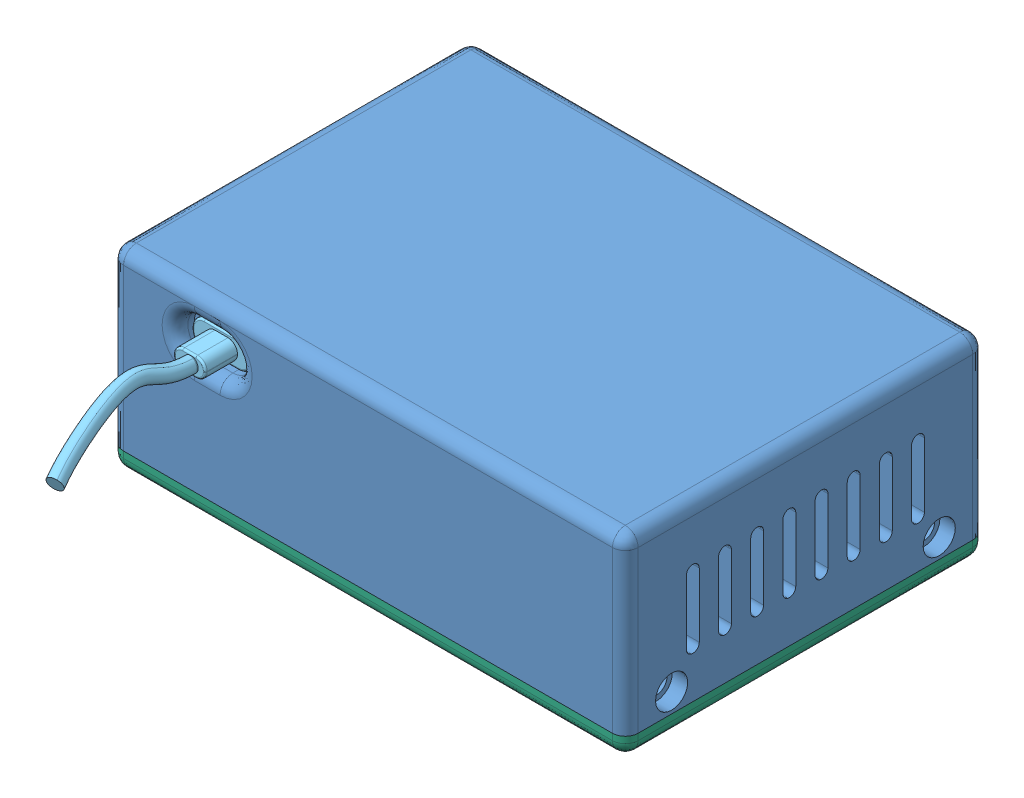
SolidWorks assembly Assem1, configuration Default. Lengths in mm.
Overall size (80 33.5 85.08).
8 component instances, 6 part files, 17 mates.
Components (placement in the parent):
- Box001-1: Box001 [Default] at (21.4141 49.2223 52.8723) x (-1 0 0) z (0 0 -1) size (80 27 56)
- raszero-1: raszero [Default] at (17.9141 46.7223 42.8723) x (-1 0 0) z (0 0 1) size (66 10.92 31.01)
- led-1: led [Default] at (1.4141 32.7223 32.8723) x (1 0 0) z (0 1 0) size (5 20 5)
- led-2: led [Default] at (21.4141 32.7223 32.8723) x (1 0 0) z (0 1 0) size (5 20 5)
- led-3: led [Default] at (41.4141 32.7223 32.8723) x (1 0 0) z (0 1 0) size (5 20 5)
- cam-1: cam [Default] at (18.4141 31.7223 52.8723) x (1 0 0) z (0 0 -1) size (58 9.5 21)
- coiled USB cable.step-1: coiled USB cable.step [Default] at (-1.6822 47.9835 115.5077) x (0.756002 -0.65305 0.044565) z (0.036289 0.109793 0.993292) size (11.86 9.41 54.78)
- Box002-3: Box002 [Default] at (31.3003 25.2223 38.2328) x (1 0 0) z (0 0 -1) size (80 9 56)
Mates (geometry in assembly coordinates):
- Coincident6: coincident aligned: plane of Box001-1 through (61.4141 52.2223 24.8723) normal (0 0 -1); circle of led-1
- Coincident7: coincident aligned: plane of Box001-1 through (61.4141 52.2223 24.8723) normal (0 0 -1); circle of led-2
- Coincident8: coincident aligned: plane of Box001-1 through (61.4141 52.2223 24.8723) normal (0 0 -1); circle of led-3
- Coincident10: coincident anti-aligned: plane of Box001-1 through (58.4141 25.2223 27.8723) normal (0 0 1); plane of raszero-1 through (-11.5859 46.2223 27.8723) normal (0 0 -1)
- Tangent1: tangent: plane of assembly; face of raszero-1; plane of coiled USB cable.step-1 through (-0.8024 45.8723 64.7223) normal (0 1 0)
- Tangent2: tangent: plane of assembly; face of raszero-1; plane of coiled USB cable.step-1 through (-0.0774 44.0223 64.7223) normal (1 0 0)
- Tangent3: tangent: plane of assembly; face of raszero-1; plane of coiled USB cable.step-1 through (-3.5024 48.8517 54.7223) normal (0 0 -1)
- Concentric1: concentric anti-aligned: cylinder of Box001-1 through (41.4141 32.7223 34.8723) axis (0 0 -1) radius 2.5; cylinder of led-3 through (41.4141 32.7223 24.8723) axis (0 0 1) radius 2.5
- Concentric2: concentric anti-aligned: cylinder of Box001-1 through (21.4141 32.7223 34.8723) axis (0 0 -1) radius 2.5; cylinder of led-2 through (21.4141 32.7223 24.8723) axis (0 0 1) radius 2.5
- Concentric3: concentric anti-aligned: cylinder of Box001-1 through (1.4141 32.7223 34.8723) axis (0 0 -1) radius 2.5; cylinder of led-1 through (1.4141 32.7223 24.8723) axis (0 0 1) radius 2.5
- Coincident14: coincident anti-aligned: plane of Box001-1 through (-15.5859 25.2223 27.8723) normal (1 0 0); plane of raszero-1 through (-15.5859 46.2023 42.8723) normal (-1 0 0)
- Coincident19: coincident aligned: plane of cam-1 through (1.4141 22.2223 52.8723) normal (0 -1 0); plane of Box002-3 through (59.4141 22.2223 26.8723) normal (0 -1 0)
- Concentric4: concentric aligned: cylinder of cam-1 through (1.4141 22.2223 52.8723) axis (0 1 0) radius 6; cylinder of Box002-3 through (1.4141 22.2223 52.8723) axis (0 1 0) radius 6.5
- Parallel1: parallel anti-aligned: plane of cam-1 through (-0.5859 30.2223 63.3723) normal (0 0 1); plane of Box002-3 through (-14.5859 28.2223 76.8723) normal (0 0 -1)
- Coincident21: coincident aligned: plane of Box001-1 through (61.4141 52.2223 80.8723) normal (1 0 0); plane of Box002-3 through (61.4141 22.2223 78.8723) normal (1 0 0)
- Coincident22: coincident: plane of Box001-1 through (61.4141 52.2223 24.8723) normal (0 0 -1); line of Box002-3 through (59.4141 24.2223 24.8723) axis (-1 0 0)
- Coincident23: coincident anti-aligned: plane of Box001-1 through (21.4141 25.2223 52.8723) normal (0 -1 0); plane of Box002-3 through (59.4141 25.2223 26.8723) normal (0 1 0)
